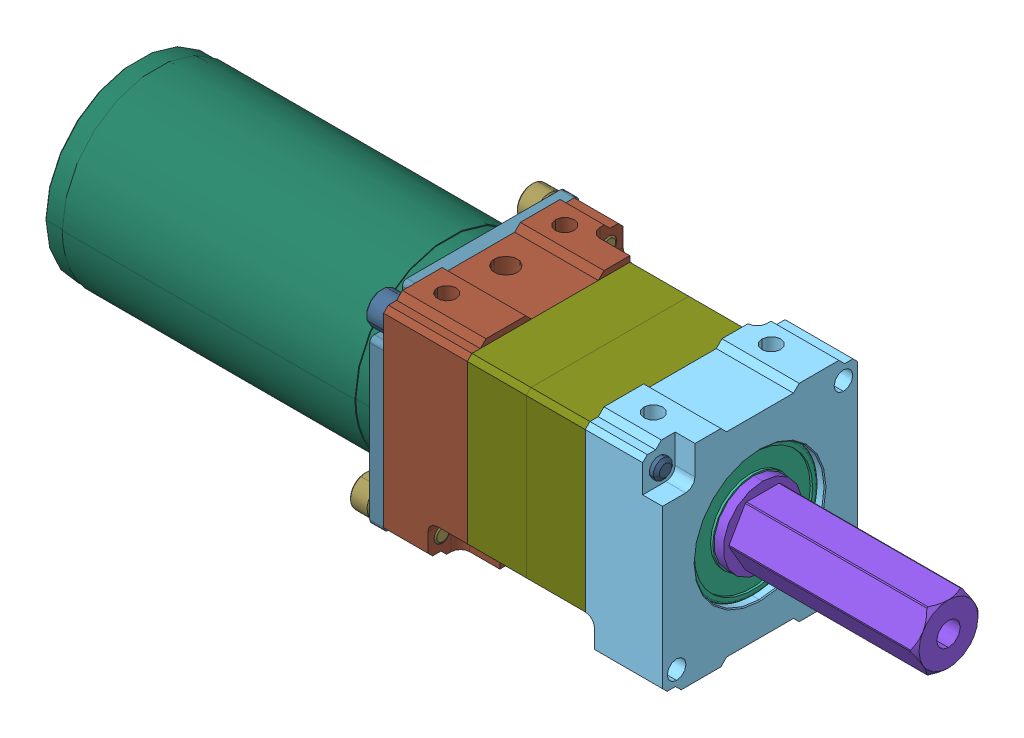
SolidWorks assembly BAG with 2-stage VersaPlanetary, configuration Default. Lengths in mm.
Overall size (176.1 63.52 63.52).
41 component instances, 19 part files, 0 mates.
Components (placement in the parent):
- VersaPlanetary v2 Two Stage 100 1 with BAG .step-1: VersaPlanetary v2 Two Stage 100 1 with BAG .step [Default] at origin size (176.1 63.52 63.52)
  - 217-2820 Rev1_Public.step-1: 217-2820 Rev1_Public.step [Default] at (-4.6546 22.225 0) x (0 -0.456494 0.889726) z (-1 0 0) size (39.22 38.88 17.4)
    - 217-2625-100.step-1: 217-2625-100.step [Default] at origin size (39.22 38.88 12.7)
      - 217-2625-008 Rev1.step-1: 217-2625-008 Rev1.step [Default] at origin size (34.7 34.7 4.7)
      - 217-2625-010 Rev1.step-1: 217-2625-010 Rev1.step [Default] at (0 10.193 3.65) x (0.999813 0.019336 0) z (0 0 1) size (4 4 12)
      - 217-2625-010 Rev1.step-2: 217-2625-010 Rev1.step [Default] at (8.691 -5.3258 3.65) size (4 4 12)
      - 217-2625-010 Rev1.step-3: 217-2625-010 Rev1.step [Default] at (-8.691 -5.3258 3.65) size (4 4 12)
      - 217-2625-005 Rev1_Planet_Revolving_Follower01.step-1: 217-2625-005 Rev1_Planet_Revolving_Follower01.step [Default] at (8.691 -5.3258 6.35) x (0.932816 0.360354 0) z (0 0 1) size (16.89 16.89 8)
      - 217-2625-005 Rev1_Planet_Revolving_Follower01.step-2: 217-2625-005 Rev1_Planet_Revolving_Follower01.step [Default] at (-8.691 -5.3258 6.35) x (-0.932788 -0.360426 0) z (0 0 1) size (16.89 16.89 8)
      - 217-2625-005 Rev1_Planet_Revolving_Follower01.step-3: 217-2625-005 Rev1_Planet_Revolving_Follower01.step [Default] at (0 10.193 6.35) x (0.893583 0.448898 0) z (0 0 1) size (16.89 16.89 8)
    - 217-2625-007 Rev1_Public.step-1: 217-2625-007 Rev1_Public.step [Default] at (0 0 6.7) x (0.992772 0.120019 0) z (0 0 1) size (15.27 15.27 12.7)
  - 217-2820 Rev1_Public.step-2: 217-2820 Rev1_Public.step [Default] at (-17.15 22.225 0) x (0 0.184082 0.982911) z (-1 0 0) size (39.22 38.88 17.4)
    - 217-2625-100.step-1: 217-2625-100.step [Default] at origin size (39.22 38.88 12.7)
      - 217-2625-008 Rev1.step-1: 217-2625-008 Rev1.step [Default] at origin size (34.7 34.7 4.7)
      - 217-2625-010 Rev1.step-1: 217-2625-010 Rev1.step [Default] at (0 10.193 3.65) x (0.999813 0.019336 0) z (0 0 1) size (4 4 12)
      - 217-2625-010 Rev1.step-2: 217-2625-010 Rev1.step [Default] at (8.691 -5.3258 3.65) size (4 4 12)
      - 217-2625-010 Rev1.step-3: 217-2625-010 Rev1.step [Default] at (-8.691 -5.3258 3.65) size (4 4 12)
      - 217-2625-005 Rev1_Planet_Revolving_Follower01.step-1: 217-2625-005 Rev1_Planet_Revolving_Follower01.step [Default] at (8.691 -5.3258 6.35) x (0.932816 0.360354 0) z (0 0 1) size (16.89 16.89 8)
      - 217-2625-005 Rev1_Planet_Revolving_Follower01.step-2: 217-2625-005 Rev1_Planet_Revolving_Follower01.step [Default] at (-8.691 -5.3258 6.35) x (-0.932788 -0.360426 0) z (0 0 1) size (16.89 16.89 8)
      - 217-2625-005 Rev1_Planet_Revolving_Follower01.step-3: 217-2625-005 Rev1_Planet_Revolving_Follower01.step [Default] at (0 10.193 6.35) x (0.893583 0.448898 0) z (0 0 1) size (16.89 16.89 8)
    - 217-2625-007 Rev1_Public.step-1: 217-2625-007 Rev1_Public.step [Default] at (0 0 6.7) x (0.992772 0.120019 0) z (0 0 1) size (15.27 15.27 12.7)
  - 217-2625-026 Rev1.step-1: 217-2625-026 Rev1.step [Default] at (-6.5 22.225 0) x (0 -1 0) z (-1 0 0) size (44.45 42 18.12)
  - 217-2742-001 Rev4.step-1: 217-2742-001 Rev4.step [Default] at (0.2002 22.225 0) x (1 0 0) z (0 -0.092627 0.995701) size (7 28 28)
  - 217-2742-001 Rev4.step-2: 217-2742-001 Rev4.step [Default] at (8.2002 22.225 0) size (7 28 28)
  - 217-2625-017 Rev1_9714K61.step-1: 217-2625-017 Rev1_9714K61.step [Default] at (7.42 22.3002 -0.342) x (0 0.56703 0.823697) z (0 -0.823697 0.56703) size (28.51 4.98 27.43)
  - 217-2625-003 Rev1.step-1: 217-2625-003 Rev1.step [Default] at (7.4478 22.225 0) x (0 -1 0) z (1 0 0) size (17 17 64.11)
  - 217-2625-018 Rev1_98541A410.step-1: 217-2625-018 Rev1_98541A410.step [Default] at (-0.7046 22.225 0) x (1 0 0) z (0 -0.017452 0.999848) size (1 19.6 17.4)
  - 832-2250-Base-Kit-Screw_SSA0832-0500ZC.step-1: 832-2250-Base-Kit-Screw_SSA0832-0500ZC.step [Default] at (-43.4 4.725 -17.5) x (0 -0.767799 -0.640691) z (0 0.640691 -0.767799) size (6.73 61.21 6.73)
  - 832-2250-Base-Kit-Screw_SSA0832-0500ZC.step-2: 832-2250-Base-Kit-Screw_SSA0832-0500ZC.step [Default] at (-43.4 39.725 17.5) x (0 0.961307 0.275478) z (0 -0.275478 0.961307) size (6.73 61.21 6.73)
  - 217-2625-025 Rev1.step-1: 217-2625-025 Rev1.step [Default] at (-35.9 22.225 0) x (0 -1 0) z (-1 0 0) size (44.45 42 18)
  - 217-4649-002 Rev1_SSA0832-0500ZC.step-1: 217-4649-002 Rev1_SSA0832-0500ZC.step [Default] at (-46.4 4.2645 17.9605) x (0 0.33842 -0.940995) z (0 0.940995 0.33842) size (6.73 16.76 6.73)
  - 217-4649-002 Rev1_SSA0832-0500ZC.step-2: 217-4649-002 Rev1_SSA0832-0500ZC.step [Default] at (-46.4 40.1855 -17.9605) x (0 -0.308932 -0.951084) z (0 0.951084 -0.308932) size (6.73 16.76 6.73)
  - 217-4649-006 Rev1_SSA0004-008BA.step-1: 217-4649-006 Rev1_SSA0004-008BA.step [Default] at (-43.4 22.225 12.5) x (0 0.5 -0.866025) z (0 -0.866025 -0.5) size (7 14 7)
  - 217-4649-006 Rev1_SSA0004-008BA.step-2: 217-4649-006 Rev1_SSA0004-008BA.step [Default] at (-43.4 22.225 -12.5) x (0 -0.5 0.866025) z (0 0.866025 0.5) size (7 14 7)
  - 217-2822-003 Rev4.step-1: 217-2822-003 Rev4.step [Default] at (-44.9 22.225 0) x (0 -1 0) z (-1 0 0) size (42 42 4.8)
  - 217-3351 Rev2.step-1: 217-3351 Rev2.step [Default] at (-46.4 22.225 0) x (0 0 1) z (1 0 0) size (59.07 59.07 84.5)
  - 217-2816-001 Rev1.step-1: 217-2816-001 Rev1.step [Default] at (-6.35 22.225 0) x (0 -1 0) z (1 0 0) size (42 42 14.51)
  - 217-2816-001 Rev1.step-2: 217-2816-001 Rev1.step [Default] at (-19.05 22.225 0) x (0 -1 0) z (1 0 0) size (42 42 14.51)
  - 217-4649-001 Rev1.step-1: 217-4649-001 Rev1.step [Default] at (-32.746 22.225 0) x (0 -1 0) z (1 0 0) size (18 18 13)
  - 217-4649-007 Rev1_94105A824.step-1: 217-4649-007 Rev1_94105A824.step [Default] at (-38.221 22.225 -6.7835) x (-0.996104 -0.088191 0) z (0 0 -1) size (4.83 4.83 4.77)
  - 217-2625-011 Rev1.step-1: 217-2625-011 Rev1.step [Default] at (-37.4818 22.225 0) x (0 0 1) z (0 -1 0) size (8.01 7.5 7.94)
